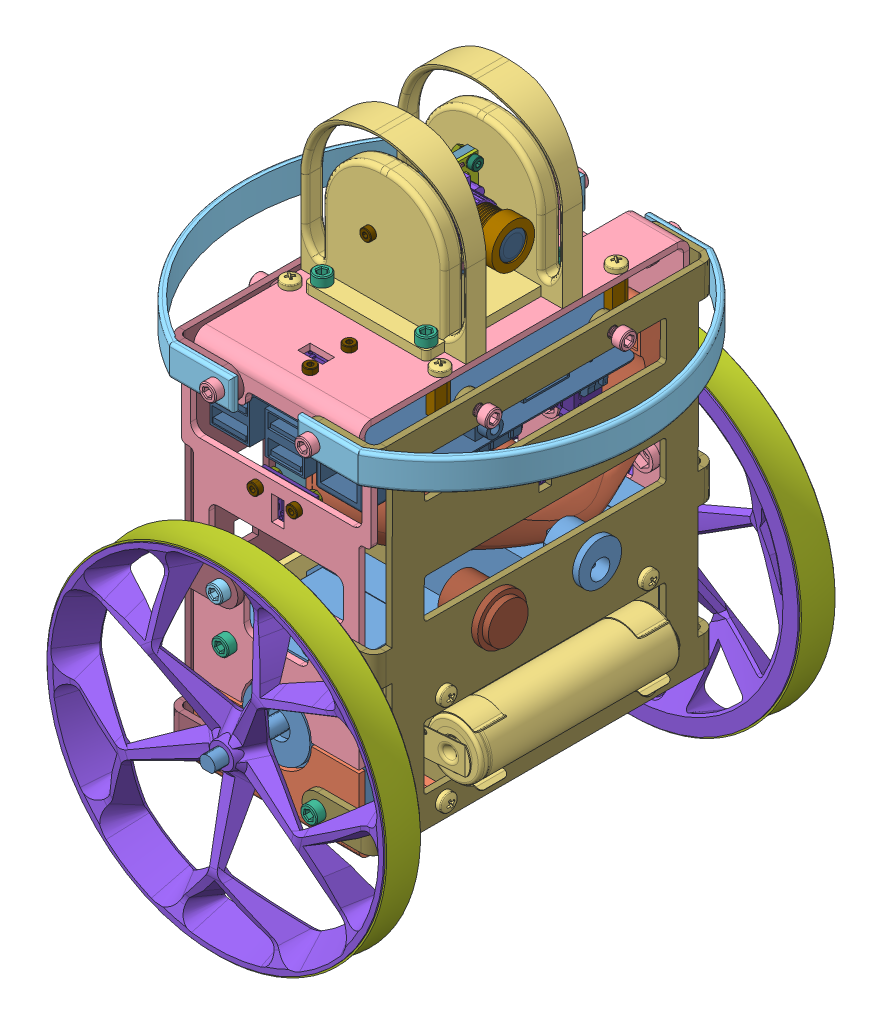
SolidWorks assembly irys5.1, configuration Domyślna. Lengths in mm.
Overall size (135.25 209.52 156.93).
165 component instances, 39 part files, 147 mates.
Components (placement in the parent):
- steppermotor-1: steppermotor [Default] at (-42.2578 -7.1789 72.25) size (42.3 42.3 64.5)
- bottomframe_rys3-1: bottomframe_rys3 [Domyślna] at (-43.1924 -30.5373 18.7182) x (0 0 -1) z (0 -1 0) size (108 54 24.86)
- steppermotor-2: steppermotor [Default] at (-42.2578 -7.1789 -31.75) x (-1 0 0) z (0 0 -1) size (42.3 42.3 64.5)
- battery_module-1: battery_module [Domyślna] at (-62.2578 -30.5373 65.25) x (0 0 -1) z (0 -1 0) size (90 40 22.7)
- topframe-1: topframe [Domyślna] at (-43.6117 88.6087 10.8622) x (0 0 -1) z (0 1 0) size (108 62 97.29)
- bumper-2: bumper [Domyślna] at (-72.7578 82.3211 20.318) x (0 0 1) z (0 -1 0) size (116 57.13 10)
- bumper-3: bumper [Domyślna] at (-11.7578 82.3211 20.25) x (0 0 1) z (0 1 0) size (116 57.13 10)
- imu-1: imu [Domyślna] at (-53.5985 -9.4799 25.3181) x (-0.019519 0 -0.999809) z (0 -1 0) size (10.16 22.86 2.23)
- camera_mounted-1: camera_mounted [Domyślna] at (-50.1687 110.2904 16.7879) x (0 0 -1) z (0.999935 0.011413 0) size (26.1 24.65 29.88)
  - Camera Module Assem-1: Camera Module Assem [Default] at (-12.4357 -13.5775 -13.0743) size (25 24 24.98)
    - PCB 1-1: PCB 1 [Default] at (8.9736 12.851 19.5114) size (25 24 2.1)
    - Camera Block-1: Camera Block [Default] at (8.9736 15.851 20.5114) size (22 13.5 12.5)
    - Camera end-1: Camera end [Default] at (8.9736 15.851 27.3922) x (0.999924 0.012337 0) z (0 0 1) size (14 14 17.26)
    - Lenz-1: Lenz [Default] at (8.9736 15.851 43.8922) size (9 9 0.5)
    - 15 Pin Ribbon Block Assem-1: 15 Pin Ribbon Block Assem [Default] at (0.7567 20.5462 10.9417) x (1 0 0) z (0 -1 0) size (22 2.5 7)
      - 15 Pin Ribbon Block-1: 15 Pin Ribbon Block [Default] at (8.217 10.8197 14.6952) size (20 2.5 6)
      - Ribbon Clamp-1: Ribbon Clamp [Default] at (8.217 10.8197 14.6952) size (22 2.5 5)
    - 0603 Resistor-1: 0603 Resistor [Default] at (2.3268 23.572 20.4882) size (1.75 0.89 0.66)
    - 0603 Resistor-2: 0603 Resistor [Default] at (4.5768 23.572 20.4882) size (1.75 0.89 0.66)
    - 0603 Resistor-3: 0603 Resistor [Default] at (15.6203 23.5707 20.4857) size (1.75 0.89 0.66)
    - 0603 Resistor-4: 0603 Resistor [Default] at (13.3703 23.5707 20.4857) size (1.75 0.89 0.66)
  - mount-1: mount [Domyślna] at (-15.8432 -12.9016 1.4371) size (25 24 5)
  - M2 x 0.4mm Thread 5mm LONG SOCKET HEAD CAP SCREW-1: M2 x 0.4mm Thread 5mm LONG SOCKET HEAD CAP SCREW [Domyślna] at (7.0379 9.2735 2.5371) x (-0.356462 0.93431 0) z (0 0 -1) size (3.8 3.8 7.09)
  - M2 x 0.4mm Thread 5mm LONG SOCKET HEAD CAP SCREW-2: M2 x 0.4mm Thread 5mm LONG SOCKET HEAD CAP SCREW [Domyślna] at (7.0379 -4.7265 2.5371) x (-0.994039 0.109029 0) z (0 0 -1) size (3.8 3.8 7.09)
  - M2 x 0.4mm Thread 5mm LONG SOCKET HEAD CAP SCREW-3: M2 x 0.4mm Thread 5mm LONG SOCKET HEAD CAP SCREW [Domyślna] at (-13.9621 9.2735 2.5371) x (-0.583934 -0.811801 0) z (0 0 -1) size (3.8 3.8 7.09)
  - M2 x 0.4mm Thread 5mm LONG SOCKET HEAD CAP SCREW-4: M2 x 0.4mm Thread 5mm LONG SOCKET HEAD CAP SCREW [Domyślna] at (-13.9621 -4.7265 2.5371) x (-0.923728 -0.383049 0) z (0 0 -1) size (3.8 3.8 7.09)
  - m2_x_0_4mm_thread_hex_nut-1: m2_x_0_4mm_thread_hex_nut [Domyślna] at (7.0379 9.2735 3.1371) size (4 4.62 1.6)
  - m2_x_0_4mm_thread_hex_nut-2: m2_x_0_4mm_thread_hex_nut [Domyślna] at (7.0379 -4.7265 3.1371) size (4 4.62 1.6)
  - m2_x_0_4mm_thread_hex_nut-3: m2_x_0_4mm_thread_hex_nut [Domyślna] at (-13.9621 -4.7265 3.1371) size (4 4.62 1.6)
  - m2_x_0_4mm_thread_hex_nut-4: m2_x_0_4mm_thread_hex_nut [Domyślna] at (-13.9621 9.2735 3.1371) size (4 4.62 1.6)
- ToF_nut-3: ToF_nut [Domyślna] at (-29.7647 53.9524 20.8423) x (0 1 0) z (1 0 0) size (12.89 18.5 4.22)
  - vl53l1x-1: vl53l1x [Domyślna] at (-6.7913 -9.4823 16.6745) size (12.7 17.78 2.22)
  - m2_x_0_4mm_thread_hex_nut-1: m2_x_0_4mm_thread_hex_nut [Domyślna] at (3.3687 5.7577 15.8745) size (4 4.62 1.6)
  - m2_x_0_4mm_thread_hex_nut-2: m2_x_0_4mm_thread_hex_nut [Domyślna] at (3.3687 -6.9423 15.8745) x (-0.923728 -0.383049 0) z (0 0 -1) size (4 4.62 1.6)
  - m2_x_0_4mm_thread_hex_nut-3: m2_x_0_4mm_thread_hex_nut [Domyślna] at (3.3687 5.7577 18.4945) x (-0.923728 -0.383049 0) z (0 0 -1) size (4 4.62 1.6) (hidden)
  - m2_x_0_4mm_thread_hex_nut-4: m2_x_0_4mm_thread_hex_nut [Domyślna] at (3.3687 -6.9423 18.4945) x (-0.923728 -0.383049 0) z (0 0 -1) size (4 4.62 1.6) (hidden)
- m2_x_0_4mm_thread_6mm_long_sock-3: m2_x_0_4mm_thread_6mm_long_sock [Domyślna] at (-14.4701 57.3211 13.9) x (0 0.924225 0.381849) z (-1 0 0) size (3.8 3.8 8)
- m2_x_0_4mm_thread_6mm_long_sock-5: m2_x_0_4mm_thread_6mm_long_sock [Domyślna] at (-14.4701 57.3211 26.6) x (0 0.924225 0.381849) z (-1 0 0) size (3.8 3.8 8)
- ToF_nut-5: ToF_nut [Domyślna] at (-42.1264 69.3142 59.6577) x (1 0 0) z (0 1 0) size (12.89 18.5 4.22)
  - vl53l1x-1: vl53l1x [Domyślna] at (-6.7913 -9.4823 16.6745) size (12.7 17.78 2.22)
  - m2_x_0_4mm_thread_hex_nut-1: m2_x_0_4mm_thread_hex_nut [Domyślna] at (3.3687 5.7577 15.8745) size (4 4.62 1.6)
  - m2_x_0_4mm_thread_hex_nut-2: m2_x_0_4mm_thread_hex_nut [Domyślna] at (3.3687 -6.9423 15.8745) x (-0.923728 -0.383049 0) z (0 0 -1) size (4 4.62 1.6)
  - m2_x_0_4mm_thread_hex_nut-3: m2_x_0_4mm_thread_hex_nut [Domyślna] at (3.3687 5.7577 18.4945) x (-0.923728 -0.383049 0) z (0 0 -1) size (4 4.62 1.6) (hidden)
  - m2_x_0_4mm_thread_hex_nut-4: m2_x_0_4mm_thread_hex_nut [Domyślna] at (3.3687 -6.9423 18.4945) x (-0.923728 -0.383049 0) z (0 0 -1) size (4 4.62 1.6) (hidden)
- m2_x_0_4mm_thread_6mm_long_sock-7: m2_x_0_4mm_thread_6mm_long_sock [Domyślna] at (-38.7578 84.6087 53.9) x (-0.868702 0 -0.495335) z (0 -1 0) size (3.8 3.8 8)
- ToF_nut-6: ToF_nut [Domyślna] at (-42.3452 53.9524 52.9555) x (0 1 0) z (0 0 1) size (12.89 18.5 4.22)
  - vl53l1x-1: vl53l1x [Domyślna] at (-6.7913 -9.4823 16.6745) size (12.7 17.78 2.22)
  - m2_x_0_4mm_thread_hex_nut-1: m2_x_0_4mm_thread_hex_nut [Domyślna] at (3.3687 5.7577 15.8745) size (4 4.62 1.6)
  - m2_x_0_4mm_thread_hex_nut-2: m2_x_0_4mm_thread_hex_nut [Domyślna] at (3.3687 -6.9423 15.8745) x (-0.923728 -0.383049 0) z (0 0 -1) size (4 4.62 1.6)
  - m2_x_0_4mm_thread_hex_nut-3: m2_x_0_4mm_thread_hex_nut [Domyślna] at (3.3687 5.7577 18.4945) x (-0.923728 -0.383049 0) z (0 0 -1) size (4 4.62 1.6) (hidden)
  - m2_x_0_4mm_thread_hex_nut-4: m2_x_0_4mm_thread_hex_nut [Domyślna] at (3.3687 -6.9423 18.4945) x (-0.923728 -0.383049 0) z (0 0 -1) size (4 4.62 1.6) (hidden)
- ToF_nut-7: ToF_nut [Domyślna] at (-41.1605 53.9524 -12.4555) x (0 1 0) z (0 0 -1) size (12.89 18.5 4.22)
  - vl53l1x-1: vl53l1x [Domyślna] at (-6.7913 -9.4823 16.6745) size (12.7 17.78 2.22)
  - m2_x_0_4mm_thread_hex_nut-1: m2_x_0_4mm_thread_hex_nut [Domyślna] at (3.3687 5.7577 15.8745) size (4 4.62 1.6)
  - m2_x_0_4mm_thread_hex_nut-2: m2_x_0_4mm_thread_hex_nut [Domyślna] at (3.3687 -6.9423 15.8745) x (-0.923728 -0.383049 0) z (0 0 -1) size (4 4.62 1.6)
  - m2_x_0_4mm_thread_hex_nut-3: m2_x_0_4mm_thread_hex_nut [Domyślna] at (3.3687 5.7577 18.4945) x (-0.923728 -0.383049 0) z (0 0 -1) size (4 4.62 1.6) (hidden)
  - m2_x_0_4mm_thread_hex_nut-4: m2_x_0_4mm_thread_hex_nut [Domyślna] at (3.3687 -6.9423 18.4945) x (-0.923728 -0.383049 0) z (0 0 -1) size (4 4.62 1.6) (hidden)
- ToF_nut-9: ToF_nut [Domyślna] at (-54.7508 53.9524 -12.3215) x (0 1 0) z (-1 0 0) size (12.89 18.5 4.22)
  - vl53l1x-1: vl53l1x [Domyślna] at (-6.7913 -9.4823 16.6745) size (12.7 17.78 2.22)
  - m2_x_0_4mm_thread_hex_nut-1: m2_x_0_4mm_thread_hex_nut [Domyślna] at (3.3687 5.7577 15.8745) size (4 4.62 1.6)
  - m2_x_0_4mm_thread_hex_nut-2: m2_x_0_4mm_thread_hex_nut [Domyślna] at (3.3687 -6.9423 15.8745) x (-0.923728 -0.383049 0) z (0 0 -1) size (4 4.62 1.6)
  - m2_x_0_4mm_thread_hex_nut-3: m2_x_0_4mm_thread_hex_nut [Domyślna] at (3.3687 5.7577 18.4945) x (-0.923728 -0.383049 0) z (0 0 -1) size (4 4.62 1.6) (hidden)
  - m2_x_0_4mm_thread_hex_nut-4: m2_x_0_4mm_thread_hex_nut [Domyślna] at (3.3687 -6.9423 18.4945) x (-0.923728 -0.383049 0) z (0 0 -1) size (4 4.62 1.6) (hidden)
- m2_x_0_4mm_thread_6mm_long_sock-11: m2_x_0_4mm_thread_6mm_long_sock [Domyślna] at (-69.6779 57.3211 -18.0792) x (0 -0.924225 -0.381849) z (1 0 0) size (3.8 3.8 8)
- m2_x_0_4mm_thread_6mm_long_sock-12: m2_x_0_4mm_thread_6mm_long_sock [Domyślna] at (-69.902 57.3211 -5.3792) x (0 -0.924225 -0.381849) z (1 0 0) size (3.8 3.8 8)
- m2_x_0_4mm_thread_6mm_long_sock-15: m2_x_0_4mm_thread_6mm_long_sock [Domyślna] at (-48.1029 57.3211 68.25) x (-0.262854 -0.964836 0) z (0 0 -1) size (3.8 3.8 8)
- m2_x_0_4mm_thread_6mm_long_sock-16: m2_x_0_4mm_thread_6mm_long_sock [Domyślna] at (-35.4029 57.3211 68.25) x (0.638921 -0.769272 0) z (0 0 -1) size (3.8 3.8 8)
- m2_x_0_4mm_thread_6mm_long_sock-17: m2_x_0_4mm_thread_6mm_long_sock [Domyślna] at (-48.1029 57.3211 -27.75) size (3.8 3.8 8)
- m2_x_0_4mm_thread_6mm_long_sock-18: m2_x_0_4mm_thread_6mm_long_sock [Domyślna] at (-35.9963 57.335 -27.7658) size (3.8 3.8 8)
- H-H_M3x12mm-1: H-H_M3x12mm [Predeterminado] at (-51.2078 -22.4959 17.65) x (0.837169 0 0.546944) z (0.546944 0 -0.837169) size (5.77 12 5)
- H-H_M3x6mm-1: H-H_M3x6mm [Predeterminado] at (-51.2078 -13.4959 17.65) x (0.837169 0 0.546944) z (0.546944 0 -0.837169) size (5.77 6 5)
- pan cross head_am-2: pan cross head_am [B18.6.7M - M3 x 0.5 x 6 Type I Cross Recessed PHMS --6N] at (-51.2078 -7.0799 17.65) x (0 -1 0) z (0 0 1) size (8.37 5.6 5.6)
- battery_module_H-2: battery_module_H [Domyślna] at (13.655 -6.0808 19.8906) x (0 0 1) z (-1 0 0) size (90 40 24.06)
  - battery_module-1: battery_module [Domyślna] at (-44.6406 -21.0981 81.7004) size (90 40 22.7)
  - H-H_M3x6mm-1: H-H_M3x6mm [Predeterminado] at (-32.6406 13.9019 84.7004) x (1 0 0) z (0 1 0) size (5.77 6 5)
  - H-H_M3x6mm-2: H-H_M3x6mm [Predeterminado] at (33.3594 13.9019 84.7004) x (1 0 0) z (0 1 0) size (5.77 6 5)
  - H-H_M3x6mm-3: H-H_M3x6mm [Predeterminado] at (-32.6406 -16.0981 84.7004) x (1 0 0) z (0 -1 0) size (5.77 6 5)
  - H-H_M3x6mm-4: H-H_M3x6mm [Predeterminado] at (33.3594 -16.0981 84.7004) x (1 0 0) z (0 1 0) size (5.77 6 5)
  - pan cross head_am-1: pan cross head_am [B18.6.7M - M3 x 0.5 x 6 Type I Cross Recessed PHMS --6N] at (-32.6406 -16.0981 77.2589) x (0 0 1) z (-1 0 0) size (8.37 5.6 5.6)
  - pan cross head_am-3: pan cross head_am [B18.6.7M - M3 x 0.5 x 6 Type I Cross Recessed PHMS --6N] at (-32.6406 13.9019 77.2589) x (0 0 1) z (-1 0 0) size (8.37 5.6 5.6)
  - pan cross head_am-4: pan cross head_am [B18.6.7M - M3 x 0.5 x 6 Type I Cross Recessed PHMS --6N] at (33.3594 13.9019 77.2589) x (0 0 1) z (-1 0 0) size (8.37 5.6 5.6)
  - pan cross head_am-5: pan cross head_am [B18.6.7M - M3 x 0.5 x 6 Type I Cross Recessed PHMS --6N] at (33.3594 -16.0981 77.2589) x (0 0 1) z (-1 0 0) size (8.37 5.6 5.6)
- pan cross head_am-3: pan cross head_am [B18.6.7M - M3 x 0.5 x 6 Type I Cross Recessed PHMS --6N] at (-78.4454 -22.1789 53.25) size (8.37 5.6 5.6)
- pan cross head_am-4: pan cross head_am [B18.6.7M - M3 x 0.5 x 6 Type I Cross Recessed PHMS --6N] at (-78.4454 7.8211 53.25) size (8.37 5.6 5.6)
- pan cross head_am-5: pan cross head_am [B18.6.7M - M3 x 0.5 x 6 Type I Cross Recessed PHMS --6N] at (-78.4454 7.8211 -12.75) size (8.37 5.6 5.6)
- pan cross head_am-6: pan cross head_am [B18.6.7M - M3 x 0.5 x 6 Type I Cross Recessed PHMS --6N] at (-78.4454 -22.1789 -12.75) size (8.37 5.6 5.6)
- pan cross head_am-7: pan cross head_am [B18.6.7M - M3 x 0.5 x 6 Type I Cross Recessed PHMS --6N] at (-57.2578 -34.9373 53.25) x (0 1 0) z (0 0 1) size (8.37 5.6 5.6)
- pan cross head_am-8: pan cross head_am [B18.6.7M - M3 x 0.5 x 6 Type I Cross Recessed PHMS --6N] at (-27.2578 -34.9373 53.25) x (0 1 0) z (0 0 1) size (8.37 5.6 5.6)
- pan cross head_am-9: pan cross head_am [B18.6.7M - M3 x 0.5 x 6 Type I Cross Recessed PHMS --6N] at (-57.2578 -34.9373 -12.75) x (0 1 0) z (0 0 1) size (8.37 5.6 5.6)
- pan cross head_am-10: pan cross head_am [B18.6.7M - M3 x 0.5 x 6 Type I Cross Recessed PHMS --6N] at (-27.2578 -34.9373 -12.75) x (0 1 0) z (0 0 1) size (8.37 5.6 5.6)
- battery_module_H-3: battery_module_H [Domyślna] at (-98.1705 -8.277 19.8906) x (0 0 1) z (1 0 0) size (90 40 24.06)
  - battery_module-1: battery_module [Domyślna] at (-44.6406 -21.0981 81.7004) size (90 40 22.7)
  - H-H_M3x6mm-1: H-H_M3x6mm [Predeterminado] at (-32.6406 13.9019 84.7004) x (1 0 0) z (0 1 0) size (5.77 6 5)
  - H-H_M3x6mm-2: H-H_M3x6mm [Predeterminado] at (33.3594 13.9019 84.7004) x (1 0 0) z (0 1 0) size (5.77 6 5)
  - H-H_M3x6mm-3: H-H_M3x6mm [Predeterminado] at (-32.6406 -16.0981 84.7004) x (1 0 0) z (0 -1 0) size (5.77 6 5)
  - H-H_M3x6mm-4: H-H_M3x6mm [Predeterminado] at (33.3594 -16.0981 84.7004) x (1 0 0) z (0 1 0) size (5.77 6 5)
  - pan cross head_am-1: pan cross head_am [B18.6.7M - M3 x 0.5 x 6 Type I Cross Recessed PHMS --6N] at (-32.6406 -16.0981 77.2589) x (0 0 1) z (-1 0 0) size (8.37 5.6 5.6)
  - pan cross head_am-3: pan cross head_am [B18.6.7M - M3 x 0.5 x 6 Type I Cross Recessed PHMS --6N] at (-32.6406 13.9019 77.2589) x (0 0 1) z (-1 0 0) size (8.37 5.6 5.6)
  - pan cross head_am-4: pan cross head_am [B18.6.7M - M3 x 0.5 x 6 Type I Cross Recessed PHMS --6N] at (33.3594 13.9019 77.2589) x (0 0 1) z (-1 0 0) size (8.37 5.6 5.6)
  - pan cross head_am-5: pan cross head_am [B18.6.7M - M3 x 0.5 x 6 Type I Cross Recessed PHMS --6N] at (33.3594 -16.0981 77.2589) x (0 0 1) z (-1 0 0) size (8.37 5.6 5.6)
- pan cross head_am-11: pan cross head_am [B18.6.7M - M3 x 0.5 x 6 Type I Cross Recessed PHMS --6N] at (-6.0701 -22.1789 53.25) x (-1 0 0) z (0 0.924225 0.381849) size (8.37 5.6 5.6)
- pan cross head_am-12: pan cross head_am [B18.6.7M - M3 x 0.5 x 6 Type I Cross Recessed PHMS --6N] at (-6.0701 7.8211 53.25) x (-1 0 0) z (0 0.924225 0.381849) size (8.37 5.6 5.6)
- pan cross head_am-13: pan cross head_am [B18.6.7M - M3 x 0.5 x 6 Type I Cross Recessed PHMS --6N] at (-6.0701 7.8211 -12.75) x (-1 0 0) z (0 0.924225 0.381849) size (8.37 5.6 5.6)
- pan cross head_am-14: pan cross head_am [B18.6.7M - M3 x 0.5 x 6 Type I Cross Recessed PHMS --6N] at (-6.0701 -22.1789 -12.75) x (-1 0 0) z (0 0.924225 0.381849) size (8.37 5.6 5.6)
- M3x6-1: M3x6 [Default] at (-57.7578 82.3211 -40.75) x (0 0 1) z (0.923728 0.383049 0) size (9 5.5 5.5)
- M3x6-2: M3x6 [Default] at (-26.7578 82.3211 -40.75) x (0 0 1) z (0.923728 0.383049 0) size (9 5.5 5.5)
- M3x4-1: M3x4 [Default] at (-26.7578 24.3211 -38.75) x (0 0 1) z (0.923728 0.383049 0) size (7 5.5 5.5)
- M3x4-2: M3x4 [Default] at (-57.7578 24.3211 -38.75) x (0 0 1) z (0.923728 0.383049 0) size (7 5.5 5.5)
- M3x8-1: M3x8 [Default] at (-26.7578 8.3211 -36.75) x (0 0 1) z (0.923728 0.383049 0) size (9 5.5 5.5)
- M3x8-2: M3x8 [Default] at (-57.7578 8.3211 -36.75) x (0 0 1) z (0.923728 0.383049 0) size (9 5.5 5.5)
- M3x8-3: M3x8 [Default] at (-26.7578 -22.6789 -38.75) x (0 0 1) z (-0.923728 -0.383049 0) size (9 5.5 5.5)
- M3x8-4: M3x8 [Default] at (-57.7578 -22.6789 -38.75) x (0 0 1) z (0.923728 0.383049 0) size (9 5.5 5.5)
- M3x6-3: M3x6 [Default] at (-57.7578 82.3211 81.318) x (0 0 -1) z (-0.923728 -0.383049 0) size (9 5.5 5.5)
- M3x6-4: M3x6 [Default] at (-26.7578 82.3211 81.25) x (0 0 -1) z (-0.923728 -0.383049 0) size (9 5.5 5.5)
- M3x4-3: M3x4 [Default] at (-57.7578 24.3211 79.25) x (0 0 -1) z (-0.923728 -0.383049 0) size (7 5.5 5.5)
- M3x4-4: M3x4 [Default] at (-26.7578 24.3211 79.25) x (0 0 -1) z (-0.923728 -0.383049 0) size (7 5.5 5.5)
- M3x8-5: M3x8 [Default] at (-57.7578 8.3211 77.25) x (0 0 -1) z (-0.923728 -0.383049 0) size (9 5.5 5.5)
- M3x8-6: M3x8 [Default] at (-26.7578 8.3211 77.25) x (0 0 -1) z (-0.923728 -0.383049 0) size (9 5.5 5.5)
- M3x8-7: M3x8 [Default] at (-57.7578 -22.6789 79.25) x (0 0 -1) z (-0.923728 -0.383049 0) size (9 5.5 5.5)
- M3x8-8: M3x8 [Default] at (-26.7578 -22.6789 79.25) x (0 0 -1) z (-0.923728 -0.383049 0) size (9 5.5 5.5)
- wheel_module-1: wheel_module [Domyślna] at (-153.2578 -13.8345 -56.9103) x (0 0 1) z (1 0 0) size (16.77 112.94 112.94)
  - tire wide-1: tire wide [Domyślna] at (-0.6464 -6.6556 111) size (11 111 111)
  - wheel_rim_minirys-1: wheel_rim_minirys [Domyślna] at (15.6603 -6.6556 111) x (0 0.027139 0.999632) z (-1 0 0) size (110 110 16.77)
- wheel_module-2: wheel_module [Domyślna] at (-153.4368 -5.0545 97.8035) x (0 0 -1) z (0.999168 0.040772 0) size (16.77 112.94 112.94)
  - tire wide-1: tire wide [Domyślna] at (-0.6464 -6.6556 111) size (11 111 111)
  - wheel_rim_minirys-1: wheel_rim_minirys [Domyślna] at (15.6603 -6.6556 111) x (0 0.027139 0.999632) z (-1 0 0) size (110 110 16.77)
- m2_x_0_4mm_thread_6mm_long_sock-19: m2_x_0_4mm_thread_6mm_long_sock [Domyślna] at (-38.7578 84.6087 66.6) x (-0.868702 0 -0.495335) z (0 -1 0) size (3.8 3.8 8)
- M3x6-5: M3x6 [Default] at (-80.7156 82.8211 -1.75) x (1 0 0) z (0 -0.999999 0.001298) size (9 5.5 5.5)
- M3x6-6: M3x6 [Default] at (-80.685 82.8211 42.25) x (1 0 0) z (0 -0.999999 0.001298) size (9 5.5 5.5)
- M3x6-7: M3x6 [Default] at (-3.0454 82.8211 42.25) x (-1 0 0) z (0 -0.383049 0.923728) size (9 5.5 5.5)
- M3x6-8: M3x6 [Default] at (-3.0454 82.8211 -1.75) x (-1 0 0) z (0 -0.383049 0.923728) size (9 5.5 5.5)
- H-M_M3x10x6mm-1: H-M_M3x10x6mm [Predeterminado] at (-66.7578 78.6087 45.25) size (5.77 16 5)
- H-M_M3x10x6mm-2: H-M_M3x10x6mm [Predeterminado] at (-18.2481 78.6087 45.3511) size (5.77 16 5)
- H-M_M3x10x6mm-5: H-M_M3x10x6mm [Predeterminado] at (-66.7578 78.6087 -12.7875) size (5.77 16 5)
- H-M_M3x10x6mm-6: H-M_M3x10x6mm [Predeterminado] at (-18.2481 78.6087 -12.6864) size (5.77 16 5)
- rys_PCB_rpi_simple-2: rys_PCB_rpi_simple [Domyślna] at (-94.7865 65.3087 -58.1904) x (1 0 0) z (0 -1 0) size (61.22 87.74 23.25)
- pan cross head_am-15: pan cross head_am [B18.6.7M - M3 x 0.5 x 6 Type I Cross Recessed PHMS --6N] at (-66.7578 93.0087 45.25) x (0 -1 0) z (-0.546944 0 0.837169) size (8.37 5.6 5.6)
- pan cross head_am-16: pan cross head_am [B18.6.7M - M3 x 0.5 x 6 Type I Cross Recessed PHMS --6N] at (-18.1875 93.0087 -12.75) x (0 -1 0) z (-0.546944 0 0.837169) size (8.37 5.6 5.6)
- pan cross head_am-17: pan cross head_am [B18.6.7M - M3 x 0.5 x 6 Type I Cross Recessed PHMS --6N] at (-66.7578 93.0087 -12.75) x (0 -1 0) z (-0.546944 0 0.837169) size (8.37 5.6 5.6)
- pan cross head_am-18: pan cross head_am [B18.6.7M - M3 x 0.5 x 6 Type I Cross Recessed PHMS --6N] at (-17.7578 93.0087 45.25) x (0 -1 0) z (-0.546944 0 0.837169) size (8.37 5.6 5.6)
- switch_simple-1: switch_simple [Domyślna] at (-4.4701 21.3211 36.25) x (0 0 1) z (-1 0 0) size (16 16 16)
- frontv5-4: frontv5 [Domyślna] at (-10.3534 69.423 20.4236) x (0 0 -1) z (-0.002586 -0.999997 0) size (112 23.29 115)
- frontv2.1-1: frontv2.1 [Domyślna] at (-74.0454 69.4652 20.0972) x (0 0 1) z (0 -1 0) size (112 23.29 115)
- fan_simple_2-6: fan_simple_2 [Domyślna] at (-74.0454 35.3211 20.2708) x (0 -1 0) z (0 0 1) size (45 10 45)
- M3x20-1: M3x20 [Default] at (-79.0454 16.8211 38.7708) size (23.05 5.5 5.5)
- M3x20-2: M3x20 [Default] at (-79.0454 16.8211 1.7708) size (23.05 5.5 5.5)
- M3x20-3: M3x20 [Default] at (-79.0454 53.8211 1.7708) size (23.05 5.5 5.5)
- M3x20-4: M3x20 [Default] at (-79.0454 53.8211 38.7708) size (23.05 5.5 5.5)
- M3_NUT-1: M3_NUT [Valor predeterminado] at (-60.7954 16.8211 38.7969) x (0 0 -1) z (1 0 0) size (6.55 5.4 2.5)
- M3_NUT-2: M3_NUT [Valor predeterminado] at (-60.9756 16.7949 1.797) x (0 0 -1) z (1 0 0) size (6.55 5.4 2.5)
- M3_NUT-3: M3_NUT [Valor predeterminado] at (-60.8582 53.7949 1.7708) x (0 0 -1) z (1 0 0) size (6.55 5.4 2.5)
- M3_NUT-4: M3_NUT [Valor predeterminado] at (-60.7954 53.8211 38.7708) x (0 0 -1) z (1 0 0) size (6.55 5.4 2.5)
- 430250200.stp-4: 430250200.stp [Domyślna] at (-24.9794 51.5777 -9.5364) x (-0.999962 0 -0.008727) z (0.008727 0 -0.999962) size (5.28 14 10.85)
- 430250200.stp-5: 430250200.stp [Domyślna] at (-40.3519 51.7087 -9.9151) x (-0.999962 0 -0.008727) z (0.008727 0 -0.999962) size (5.28 14 10.85)
- 430250200.stp-6: 430250200.stp [Domyślna] at (-47.7794 51.7087 -9.6936) x (-0.999962 0 -0.008727) z (0.008727 0 -0.999962) size (5.28 14 10.85)
- 430250200.stp-7: 430250200.stp [Domyślna] at (-31.8678 51.7087 -9.7603) x (-0.999962 0 -0.008727) z (0.008727 0 -0.999962) size (5.28 14 10.85)
- M2 x 0.4mm Thread 10mm LONG SOCKET HEAD CAP SCREW-5: M2 x 0.4mm Thread 10mm LONG SOCKET HEAD CAP SCREW [Domyślna] at (-46.2578 112.6087 11.25) x (-0.266188 0.963921 0) z (0 0 1) size (3.8 3.8 12.09)
- M2 x 0.4mm Thread 10mm LONG SOCKET HEAD CAP SCREW-6: M2 x 0.4mm Thread 10mm LONG SOCKET HEAD CAP SCREW [Domyślna] at (-46.2578 112.6087 29.25) x (-0.999935 -0.011413 0) z (0 0 -1) size (3.8 3.8 12.09)
- M3x8-9: M3x8 [Default] at (-25.2578 96.6087 -1.75) x (0 -1 0) z (-0.923728 0 0.383049) size (9 5.5 5.5)
- M3x8-13: M3x8 [Default] at (-59.2578 96.6087 42.25) x (0 -1 0) z (-0.923728 0 0.383049) size (9 5.5 5.5)
- M3x8-14: M3x8 [Default] at (-25.2578 96.6087 42.25) x (0 -1 0) z (-0.923728 0 0.383049) size (9 5.5 5.5)
- M3x8-15: M3x8 [Default] at (-59.2578 96.6087 -1.75) x (0 -1 0) z (-0.923728 0 0.383049) size (9 5.5 5.5)
- Panel_Mount_2mm_Power_Plug_v2.step-1: Panel_Mount_2mm_Power_Plug_v2.step [Domyślna] at (-6.4714 21.2686 4.25) x (0 -0.000012 -1) z (0.002586 0.999997 -0.000012) size (14 13.69 14)
- tunelv3.2-1: tunelv3.2 [Domyślna] at (-62.0454 58.4238 13.3551) x (0 -0.000707 -1) z (1 0 0) size (74.54 69.73 61.73)
- mount3-1: mount3 [Domyślna] at (-42.2578 90.6087 20.25) x (0 0 -1) z (1 0 0) size (50 53 54.12)
Mates (geometry in assembly coordinates):
- Koncentryczne1: concentric aligned: cylinder of steppermotor-1 through (-26.7578 -22.6789 64.75) axis (0 0 1) radius 1.25; cylinder of bottomframe_rys3-1 through (-26.7578 -22.6789 74.25) axis (0 0 1) radius 1.6
- Koncentryczne2: concentric aligned: cylinder of steppermotor-1 through (-57.7578 -22.6789 64.75) axis (0 0 1) radius 1.25; cylinder of bottomframe_rys3-1 through (-57.7578 -22.6789 74.25) axis (0 0 1) radius 1.6
- Wspólnie1: coincident anti-aligned: plane of steppermotor-1 through (-64.2538 -29.1749 72.25) normal (0 0 1); plane of bottomframe_rys3-1 through (-42.2578 -7.6789 72.25) normal (0 0 -1)
- Koncentryczne3: concentric aligned: cylinder of bottomframe_rys3-1 through (-57.7578 -22.6789 -33.75) axis (0 0 -1) radius 1.6; cylinder of steppermotor-2 through (-57.7578 -22.6789 -24.25) axis (0 0 -1) radius 1.25
- Koncentryczne4: concentric aligned: circle of bottomframe_rys3-1; cylinder of steppermotor-2 through (-26.7578 -22.6789 -24.25) axis (0 0 -1) radius 1.25
- Wspólnie2: coincident anti-aligned: plane of bottomframe_rys3-1 through (-42.2578 -159.6789 -31.75) normal (0 0 1); plane of steppermotor-2 through (-20.2618 -29.1749 -31.75) normal (0 0 -1)
- Koncentryczne7: concentric aligned: cylinder of steppermotor-2 through (-26.7578 8.3211 -24.25) axis (0 0 -1) radius 1.25; cylinder of topframe-1 through (-26.7578 8.3211 -33.75) axis (0 0 -1) radius 1.6
- Koncentryczne8: concentric aligned: cylinder of steppermotor-1 through (-57.7578 8.3211 64.75) axis (0 0 1) radius 1.25; cylinder of topframe-1 through (-57.7578 8.3211 74.25) axis (0 0 1) radius 1.6
- Wspólnie4: coincident anti-aligned: plane of steppermotor-1 through (-64.2538 -29.1749 72.25) normal (0 0 1); plane of topframe-1 through (-70.7578 55.8211 72.25) normal (0 0 -1)
- Koncentryczne18: concentric aligned: cylinder of bottomframe_rys3-1 through (-26.7578 -22.6789 -33.75) axis (0 0 -1) radius 1.6; cylinder of steppermotor-2 through (-26.7578 -22.6789 -24.25) axis (0 0 -1) radius 1.25
- Koncentryczne36: concentric aligned: cylinder of topframe-1 through (-57.7578 82.3211 74.25) axis (0 0 1) radius 1.6; cylinder of bumper-2 through (-57.7578 82.3211 -37.682) axis (0 0 1) radius 1.5
- Koncentryczne37: concentric aligned: cylinder of topframe-1 through (-26.7578 82.3211 74.25) axis (0 0 1) radius 1.6; cylinder of bumper-3 through (-26.7578 82.3211 -37.75) axis (0 0 1) radius 1.5
- Koncentryczne55: concentric aligned: cylinder of battery_module-1 through (-51.2078 -28.4959 17.65) axis (0 1 0) radius 1.1; cylinder of imu-1 through (-51.2078 -10.4959 17.65) axis (0 1 0) radius 1.0922
- Koncentryczne56: concentric anti-aligned: cylinder of bottomframe_rys3-1 through (-27.2578 -32.5373 53.25) axis (0 -1 0) radius 1.4; cylinder of battery_module-1 through (-27.2578 -28.4959 53.25) axis (0 1 0) radius 1.6
- Koncentryczne57: concentric anti-aligned: cylinder of bottomframe_rys3-1 through (-57.2578 -32.5373 -12.75) axis (0 -1 0) radius 1.4; cylinder of battery_module-1 through (-57.2578 -28.4959 -12.75) axis (0 1 0) radius 1.6
- Wspólnie27: coincident anti-aligned: plane of bottomframe_rys3-1 through (-42.2578 -30.5373 96.25) normal (0 1 0); plane of battery_module-1 through (-62.2578 -30.5373 65.25) normal (0 -1 0)
- Koncentryczne63: concentric aligned: cylinder of topframe-1 through (-38.7578 90.6087 4.6) axis (0 1 0) radius 1.25; cylinder of camera_mounted-1/mount1-1 through (-38.7578 90.6087 4.6) axis (0 1 0) radius 1.05
- Koncentryczne65: concentric aligned: cylinder of topframe-1 through (-38.7578 90.6087 35.9) axis (0 1 0) radius 1.25; cylinder of camera_mounted-1/mount1-1 through (-38.7578 90.6087 35.9) axis (0 1 0) radius 1.05
- Wspólnie34: coincident anti-aligned: plane of topframe-1 through (-70.7578 90.6087 105.75) normal (0 1 0); plane of camera_mounted-1/mount1-1 through (-41.7578 90.6087 2.1027) normal (0 -1 0)
- Wspólnie61: coincident anti-aligned: plane of topframe-1 through (-70.7578 88.6087 105.75) normal (0 -1 0); plane of ToF_nut-5/m2_x_0_4mm_thread_hex_nut-4 through (-37.3526 88.6087 64.7673) normal (0 1 0)
- Koncentryczne100: concentric anti-aligned: cylinder of camera_mounted-1/mount1-1 through (-38.7578 90.6087 35.9) axis (0 1 0) radius 1.05; cylinder of M2 x 0.4mm Thread 10mm LONG SOCKET HEAD CAP SCREW-4 through (-38.7578 95.6087 35.9) axis (0 -1 0) radius 1.9
- Wspólnie64: coincident anti-aligned: plane of camera_mounted-1/mount1-1 through (-41.7578 93.6087 7.7527) normal (0 1 0); plane of M2 x 0.4mm Thread 10mm LONG SOCKET HEAD CAP SCREW-4 through (-38.7578 93.6087 35.9) normal (0 -1 0)
- Koncentryczne104: concentric aligned: cylinder of topframe-1 through (-38.7578 90.6087 53.9) axis (0 1 0) radius 1.25; cylinder of m2_x_0_4mm_thread_6mm_long_sock-7 through (-38.7578 92.6087 53.9) axis (0 1 0) radius 1.9
- Wspólnie65: coincident anti-aligned: plane of topframe-1 through (-70.7578 90.6087 105.75) normal (0 1 0); plane of m2_x_0_4mm_thread_6mm_long_sock-7 through (-38.7578 90.6087 53.9) normal (0 -1 0)
- Wspólnie67: coincident anti-aligned: plane of topframe-1 through (-70.7578 55.8211 72.25) normal (0 0 -1); plane of ToF_nut-6/m2_x_0_4mm_thread_hex_nut-4 through (-37.2356 58.7262 72.25) normal (0 0 1)
- Wspólnie68: coincident anti-aligned: plane of topframe-1 through (-70.7578 226.8211 -31.75) normal (0 0 1); plane of ToF_nut-7/m2_x_0_4mm_thread_hex_nut-3 through (-33.5701 58.7262 -31.75) normal (0 0 -1)
- Wspólnie78: coincident anti-aligned: plane of topframe-1 through (-70.7578 55.8211 74.25) normal (0 0 1); plane of m2_x_0_4mm_thread_6mm_long_sock-15 through (-48.1029 57.3211 74.25) normal (0 0 -1)
- Wspólnie79: coincident anti-aligned: plane of topframe-1 through (-70.7578 55.8211 74.25) normal (0 0 1); plane of m2_x_0_4mm_thread_6mm_long_sock-16 through (-35.4029 57.3211 74.25) normal (0 0 -1)
- Wspólnie80: coincident anti-aligned: plane of topframe-1 through (-70.7578 226.8211 -33.75) normal (0 0 -1); plane of m2_x_0_4mm_thread_6mm_long_sock-17 through (-48.1029 57.3211 -33.75) normal (0 0 1)
- Koncentryczne125: concentric aligned: cylinder of battery_module-1 through (-51.2078 -28.4959 17.65) axis (0 1 0) radius 1.1; cylinder of H-H_M3x12mm-1 through (-51.2078 -28.4959 17.65) axis (0 1 0) radius 1.5
- Wspólnie82: coincident anti-aligned: plane of battery_module-1 through (-62.2578 -28.4959 65.25) normal (0 1 0); plane of H-H_M3x12mm-1 through (-51.2078 -28.4959 17.65) normal (0 -1 0)
- Wspólnie83: coincident anti-aligned: circle of H-H_M3x12mm-1; cylinder of H-H_M3x6mm-1 through (-51.2078 -16.4959 17.65) axis (0 1 0) radius 1.5
- Wspólnie84: coincident anti-aligned: plane of H-H_M3x12mm-1 through (-51.2078 -16.4959 17.65) normal (0 1 0); plane of H-H_M3x6mm-1 through (-51.2078 -16.4959 17.65) normal (0 -1 0)
- Wspólnie85: coincident anti-aligned: plane of imu-1 through (-53.5985 -10.4959 25.3181) normal (0 -1 0); plane of H-H_M3x6mm-1 through (-51.2078 -10.4959 17.65) normal (0 1 0)
- Koncentryczne1261: concentric aligned: cylinder of imu-1 through (-51.2078 -10.4959 17.65) axis (0 1 0) radius 1.0922; cylinder of pan cross head_am-2 through (-51.2078 18.3201 17.65) axis (0 1 0) radius 2.8
- Wspólnie871: coincident anti-aligned: plane of imu-1 through (-53.5985 -9.4799 25.3181) normal (0 1 0); plane of pan cross head_am-2 through (-49.7078 -9.4799 17.65) normal (0 -1 0)
- Koncentryczne1331: concentric aligned: cylinder of bottomframe_rys3-1 through (-57.2578 -32.5373 53.25) axis (0 -1 0) radius 1.4; cylinder of pan cross head_am-7 through (-57.2578 -60.3373 53.25) axis (0 -1 0) radius 2.8
- Wspólnie931: coincident anti-aligned: plane of bottomframe_rys3-1 through (-42.2578 -32.5373 96.25) normal (0 -1 0); plane of pan cross head_am-7 through (-58.7578 -32.5373 53.25) normal (0 1 0)
- Koncentryczne1341: concentric aligned: cylinder of bottomframe_rys3-1 through (-27.2578 -32.5373 53.25) axis (0 -1 0) radius 1.4; cylinder of pan cross head_am-8 through (-27.2578 -60.3373 53.25) axis (0 -1 0) radius 2.8
- Wspólnie941: coincident anti-aligned: plane of bottomframe_rys3-1 through (-42.2578 -32.5373 96.25) normal (0 -1 0); plane of pan cross head_am-8 through (-28.7578 -32.5373 53.25) normal (0 1 0)
- Koncentryczne1351: concentric aligned: cylinder of bottomframe_rys3-1 through (-57.2578 -32.5373 -12.75) axis (0 -1 0) radius 1.4; cylinder of pan cross head_am-9 through (-57.2578 -60.3373 -12.75) axis (0 -1 0) radius 2.8
- Wspólnie951: coincident anti-aligned: plane of bottomframe_rys3-1 through (-42.2578 -32.5373 96.25) normal (0 -1 0); plane of pan cross head_am-9 through (-58.7578 -32.5373 -12.75) normal (0 1 0)
- Koncentryczne1361: concentric aligned: cylinder of bottomframe_rys3-1 through (-27.2578 -32.5373 -12.75) axis (0 -1 0) radius 1.4; cylinder of pan cross head_am-10 through (-27.2578 -60.3373 -12.75) axis (0 -1 0) radius 2.8
- Wspólnie961: coincident anti-aligned: plane of bottomframe_rys3-1 through (-42.2578 -32.5373 96.25) normal (0 -1 0); plane of pan cross head_am-10 through (-28.7578 -32.5373 -12.75) normal (0 1 0)
- Wspólnie104: coincident anti-aligned: plane of bumper-3 through (-31.7578 77.3211 -37.75) normal (0 0 -1); plane of M3x6-2 through (-26.187 80.9447 -37.75) normal (0 0 1)
- Koncentryczne148: concentric aligned: cylinder of topframe-1 through (-26.7578 8.3211 -33.75) axis (0 0 -1) radius 1.6; cylinder of M3x8-1 through (-26.7578 8.3211 -125.4555) axis (0 0 -1) radius 2.75
- Wspólnie107: coincident anti-aligned: plane of topframe-1 through (-70.7578 226.8211 -33.75) normal (0 0 -1); plane of M3x8-1 through (-26.187 6.9447 -33.75) normal (0 0 1)
- Koncentryczne149: concentric aligned: cylinder of topframe-1 through (-57.7578 8.3211 -33.75) axis (0 0 -1) radius 1.6; cylinder of M3x8-2 through (-57.7578 8.3211 -125.4555) axis (0 0 -1) radius 2.75
- Wspólnie108: coincident anti-aligned: plane of topframe-1 through (-70.7578 226.8211 -33.75) normal (0 0 -1); plane of M3x8-2 through (-57.187 6.9447 -33.75) normal (0 0 1)
- Koncentryczne150: concentric aligned: cylinder of bottomframe_rys3-1 through (-57.7578 -22.6789 -33.75) axis (0 0 -1) radius 1.6; cylinder of M3x8-4 through (-57.7578 -22.6789 -127.4555) axis (0 0 -1) radius 2.75
- Koncentryczne153: concentric aligned: circle of topframe-1; cylinder of M3x6-3 through (-57.7578 82.3211 170.0235) axis (0 0 1) radius 2.75
- Wspólnie112: coincident anti-aligned: plane of bumper-2 through (-73.1394 87.3211 78.318) normal (0 0 1); plane of M3x6-3 through (-57.187 80.9447 78.318) normal (0 0 -1)
- Koncentryczne155: concentric aligned: cylinder of topframe-1 through (-57.7578 24.3211 74.25) axis (0 0 1) radius 1.6; cylinder of M3x4-3 through (-57.7578 24.3211 167.9555) axis (0 0 1) radius 2.75
- Koncentryczne158: concentric aligned: cylinder of topframe-1 through (-26.7578 8.3211 74.25) axis (0 0 1) radius 1.6; cylinder of M3x8-6 through (-26.7578 8.3211 165.9555) axis (0 0 1) radius 2.75
- Koncentryczne159: concentric aligned: cylinder of topframe-1 through (-57.7578 8.3211 74.25) axis (0 0 1) radius 1.6; cylinder of M3x8-5 through (-57.7578 8.3211 165.9555) axis (0 0 1) radius 2.75
- Wspólnie115: coincident anti-aligned: plane of topframe-1 through (-70.7578 55.8211 74.25) normal (0 0 1); plane of M3x8-5 through (-57.187 6.9447 74.25) normal (0 0 -1)
- Wspólnie116: coincident anti-aligned: plane of topframe-1 through (-70.7578 55.8211 74.25) normal (0 0 1); plane of M3x8-6 through (-26.187 6.9447 74.25) normal (0 0 -1)
- Koncentryczne1447: concentric aligned: cylinder of topframe-1 through (-48.1029 57.3211 -33.75) axis (0 0 1) radius 1.25; cylinder of ToF_nut-7/vl53l1x-1 through (-48.1029 57.3211 -30.15) axis (0 0 1) radius 1.0922
- Koncentryczne1448: concentric aligned: cylinder of topframe-1 through (-35.4029 57.3211 -33.75) axis (0 0 1) radius 1.25; cylinder of ToF_nut-7/vl53l1x-1 through (-35.4029 57.3211 -30.15) axis (0 0 1) radius 1.0922
- Równolegle1: parallel aligned: plane of ToF_nut-7/m2_x_0_4mm_thread_hex_nut-1 through (-34.2482 55.3211 -27.53) normal (0 0 1); plane of m2_x_0_4mm_thread_6mm_long_sock-18 through (-35.9963 57.335 -33.7658) normal (0 0 1)
- Koncentryczne1454: concentric aligned: circle of topframe-1; circle of ToF_nut-6/m2_x_0_4mm_thread_hex_nut-3
- Koncentryczne1455: concentric aligned: circle of topframe-1; circle of ToF_nut-6/m2_x_0_4mm_thread_hex_nut-4
- Koncentryczne1456: concentric aligned: circle of topframe-1; circle of m2_x_0_4mm_thread_6mm_long_sock-16
- Koncentryczne1457: concentric aligned: circle of topframe-1; circle of m2_x_0_4mm_thread_6mm_long_sock-15
- Koncentryczne1458: concentric aligned: circle of topframe-1; circle of m2_x_0_4mm_thread_6mm_long_sock-17
- Koncentryczne1461: concentric anti-aligned: circle of topframe-1; cylinder of ToF_nut-5/vl53l1x-1 through (-38.7578 87.0087 53.9) axis (0 -1 0) radius 1.0922
- Koncentryczne1462: concentric aligned: circle of topframe-1; circle of m2_x_0_4mm_thread_6mm_long_sock-19
- Koncentryczne1463: concentric anti-aligned: circle of bumper2-1; circle of M3x6-7
- Wspólnie970: coincident anti-aligned: plane of bumper2-1 through (-6.0454 102.864 47.0753) normal (1 0 0); plane of M3x6-7 through (-6.0454 81.4447 41.6793) normal (-1 0 0)
- Koncentryczne1464: concentric anti-aligned: circle of bumper2-2; circle of M3x6-8
- Wspólnie971: coincident anti-aligned: plane of bumper2-2 through (-6.0454 102.864 3.0753) normal (1 0 0); plane of M3x6-8 through (-6.0454 81.4447 -2.3207) normal (-1 0 0)
- Koncentryczne1465: concentric aligned: circle of bumper2-1; circle of M3x6-6
- Koncentryczne1466: concentric aligned: circle of bumper2-2; circle of M3x6-5
- Koncentryczne1483: concentric aligned: circle of H-M_M3x10x6mm-1; circle of rys_PCB_rpi_simple-2
- Wspólnie978: coincident anti-aligned: plane of H-M_M3x10x6mm-1 through (-66.7578 78.6087 45.25) normal (0 -1 0); plane of rys_PCB_rpi_simple-2 through (-42.2266 78.6087 26.4747) normal (0 1 0)
- Koncentryczne1484: concentric aligned: circle of H-M_M3x10x6mm-2; circle of rys_PCB_rpi_simple-2
- Wspólnie979: coincident anti-aligned: plane of H-M_M3x10x6mm-2 through (-18.2481 78.6087 45.3511) normal (0 -1 0); plane of rys_PCB_rpi_simple-2 through (-42.2266 78.6087 26.4747) normal (0 1 0)
- Koncentryczne1485: concentric aligned: circle of H-M_M3x10x6mm-5; circle of rys_PCB_rpi_simple-2
- Wspólnie980: coincident anti-aligned: plane of H-M_M3x10x6mm-5 through (-66.7578 78.6087 -12.7875) normal (0 -1 0); plane of rys_PCB_rpi_simple-2 through (-42.2266 78.6087 26.4747) normal (0 1 0)
- Koncentryczne1486: concentric aligned: circle of H-M_M3x10x6mm-6; circle of rys_PCB_rpi_simple-2
- Wspólnie981: coincident anti-aligned: plane of H-M_M3x10x6mm-6 through (-18.2481 78.6087 -12.6864) normal (0 -1 0); plane of rys_PCB_rpi_simple-2 through (-42.2266 78.6087 26.4747) normal (0 1 0)
- Koncentryczne1487: concentric anti-aligned: circle of topframe-1; circle of H-M_M3x10x6mm-1
- Wspólnie982: coincident anti-aligned: plane of topframe-1 through (-70.7578 88.6087 105.75) normal (0 -1 0); plane of H-M_M3x10x6mm-1 through (-66.7578 88.6087 45.25) normal (0 1 0)
- Koncentryczne1490: concentric aligned: circle of topframe-1; circle of M3X6_PLASTIC-2
- Wspólnie983: coincident aligned: plane of topframe-1 through (-70.7578 90.6087 105.75) normal (0 1 0); circle of M3X6_PLASTIC-2
- Koncentryczne1491: concentric aligned: circle of topframe-1; circle of M3X6_PLASTIC-3
- Wspólnie985: coincident aligned: plane of topframe-1 through (-70.7578 90.6087 105.75) normal (0 1 0); circle of M3X6_PLASTIC-3
- Koncentryczne1492: concentric aligned: circle of topframe-1; circle of M3X6_PLASTIC-1
- Wspólnie986: coincident aligned: plane of topframe-1 through (-70.7578 90.6087 105.75) normal (0 1 0); circle of M3X6_PLASTIC-1
- Koncentryczne1493: concentric aligned: circle of topframe-1; circle of M3X6_PLASTIC-4
- Wspólnie987: coincident aligned: plane of topframe-1 through (-70.7578 90.6087 105.75) normal (0 1 0); circle of M3X6_PLASTIC-4
- Stycznie1: tangent: circle of topframe-1; circle of front-4
- Koncentryczne1502: concentric aligned: circle of topframe-1; circle of front-4
- Koncentryczne1506: concentric aligned: circle of bottomframe_rys3-1; circle of frontv2-1
- Koncentryczne1507: concentric aligned: circle of topframe-1; circle of frontv2-1
- Koncentryczne1509: concentric aligned: circle of frontv2-1; circle of fan_simple-6
- Wspólnie1003: coincident anti-aligned: plane of frontv2.1-1 through (-74.0454 82.3211 -50.7292) normal (1 0 0); plane of fan_simple_2-6 through (-74.0454 54.8211 39.7708) normal (-1 0 0)
- Wspólnie1004: coincident anti-aligned: circle of fan_simple-6; circle of tunel-2
- Koncentryczne1514: concentric aligned: circle of frontv2-1; circle of M3x20-3
- Koncentryczne1515: concentric aligned: circle of frontv2-1; circle of M3x20-4
- Koncentryczne1516: concentric aligned: circle of frontv2-1; circle of M3x20-1
- Koncentryczne1517: concentric aligned: circle of frontv2-1; circle of M3x20-2
- Wspólnie1005: coincident anti-aligned: circle of tunel-2; circle of M3_NUT-1
- Wspólnie1006: coincident anti-aligned: circle of tunel-2; circle of M3_NUT-2
- Wspólnie1007: coincident anti-aligned: circle of tunel-2; circle of M3_NUT-4
- Wspólnie1009: coincident anti-aligned: circle of tunel-2; circle of M3_NUT-3
- Koncentryczne1518: concentric aligned: circle of steppermotor-2; circle of wheel_module-1/wheel_rim_minirys-1
- Wspólnie1010: coincident anti-aligned: plane of steppermotor-2 through (-43.8633 -9.0734 -41.25) normal (0 0 -1); plane of wheel_module-1/wheel_rim_minirys-1 through (-42.2578 -7.1789 -41.25) normal (0 0 1)
- Wspólnie1011: coincident anti-aligned: plane of frontv2.1-1 through (-76.0454 82.3211 -50.7292) normal (-1 0 0); plane of M3x20-3 through (-76.0454 55.3111 1.7708) normal (1 0 0)
- Wspólnie1012: coincident anti-aligned: plane of frontv2.1-1 through (-76.0454 82.3211 -50.7292) normal (-1 0 0); plane of M3x20-4 through (-76.0454 55.3111 38.7708) normal (1 0 0)
- Wspólnie1013: coincident anti-aligned: plane of frontv2.1-1 through (-76.0454 82.3211 -50.7292) normal (-1 0 0); plane of M3x20-1 through (-76.0454 18.3111 38.7708) normal (1 0 0)
- Wspólnie1014: coincident anti-aligned: plane of frontv2.1-1 through (-76.0454 82.3211 -50.7292) normal (-1 0 0); plane of M3x20-2 through (-76.0454 18.3111 1.7708) normal (1 0 0)
- Wspólnie1015: coincident anti-aligned: plane of topframe-1 through (-70.7578 90.6087 105.75) normal (0 1 0); plane of m2_x_0_4mm_thread_6mm_long_sock-19 through (-38.7578 90.6087 66.6) normal (0 -1 0)
- Równolegle8: parallel anti-aligned: plane of rys_PCB_rpi_simple-2 through (-27.3114 55.3587 -6.0403) normal (0 -1 0); plane of 430250200.stp-4 through (-26.9343 55.2277 -6.1233) normal (0 1 0)
- Wspólnie1024: coincident anti-aligned: plane of rys_PCB_rpi_simple-2 through (-50.9865 55.3587 -6.0153) normal (0 -1 0); plane of 430250200.stp-6 through (-49.7342 55.3587 -6.2806) normal (0 1 0)
- Wspólnie1025: coincident anti-aligned: plane of rys_PCB_rpi_simple-2 through (-43.1115 55.3587 -6.0153) normal (0 -1 0); plane of 430250200.stp-5 through (-42.3068 55.3587 -6.5021) normal (0 1 0)
- Wspólnie1026: coincident anti-aligned: plane of rys_PCB_rpi_simple-2 through (-35.2115 55.3587 -6.0153) normal (0 -1 0); plane of 430250200.stp-7 through (-33.8227 55.3587 -6.3472) normal (0 1 0)
- Koncentryczne1524: concentric aligned: circle of mount2-1; circle of M3x8-13
- Wspólnie1031: coincident anti-aligned: plane of mount2-1 through (-60.7578 93.6087 -3.25) normal (0 1 0); plane of M3x8-13 through (-58.687 93.6087 43.6264) normal (0 -1 0)
- Koncentryczne1525: concentric aligned: circle of mount2-1; circle of M3x8-14
- Koncentryczne1526: concentric aligned: circle of mount2-1; circle of M3x8-15
- Koncentryczne1527: concentric aligned: circle of mount2-1; circle of M3x8-9
- Wspólnie1032: coincident aligned: plane of mount2-1 through (-60.7578 93.6087 -3.25) normal (0 1 0); circle of M3x8-14
- Wspólnie1033: coincident aligned: plane of mount2-1 through (-60.7578 93.6087 -3.25) normal (0 1 0); circle of M3x8-15
- Wspólnie1034: coincident anti-aligned: plane of mount2-1 through (-60.7578 93.6087 -3.25) normal (0 1 0); plane of M3x8-9 through (-24.687 93.6087 -0.3736) normal (0 -1 0)
- Koncentryczne1531: concentric anti-aligned: circle of mount2-1; circle of M2 x 0.4mm Thread 10mm LONG SOCKET HEAD CAP SCREW-6
- Wspólnie1036: coincident anti-aligned: plane of mount2-1 through (-42.2578 133.6087 39.25) normal (0 0 1); plane of M2 x 0.4mm Thread 10mm LONG SOCKET HEAD CAP SCREW-6 through (-52.2578 111.1087 39.25) normal (0 0 -1)
- Koncentryczne1532: concentric anti-aligned: circle of camera_mounted-1/mount-1; circle of mount2-1
- Koncentryczne1533: concentric aligned: circle of mount2-1; circle of M2 x 0.4mm Thread 10mm LONG SOCKET HEAD CAP SCREW-5
- Wspólnie1038: coincident anti-aligned: plane of mount2-1 through (-42.2578 133.6087 1.25) normal (0 0 -1); plane of M2 x 0.4mm Thread 10mm LONG SOCKET HEAD CAP SCREW-5 through (-46.2578 111.6936 1.25) normal (0 0 1)
- Wspólnie1039: coincident anti-aligned: circle of fan_simple-6; circle of tunelv3-2
- Koncentryczne1534: concentric anti-aligned: circle of front-4; circle of Panel_Mount_2mm_Power_Plug_v2.step-1
- Wspólnie1040: coincident anti-aligned: plane of frontv5-4 through (-8.3202 82.2736 91.25) normal (0.999997 -0.002586 0); circle of Panel_Mount_2mm_Power_Plug_v2.step-1
- Wspólnie1041: coincident anti-aligned: circle of fan_simple-6; circle of tunelv3.1-1
- Wspólnie1042: coincident aligned: circle of frontv2.1-1; circle of fan_simple_2-6
- Koncentryczne1535: concentric aligned: cylinder of m2_x_0_4mm_thread_6mm_long_sock-11 through (-77.6779 57.3211 -18.0792) axis (-1 0 0) radius 1.9; circle of frontv2.1-1
- Koncentryczne1536: concentric anti-aligned: circle of m2_x_0_4mm_thread_6mm_long_sock-12; circle of frontv2.1-1
- Koncentryczne1537: concentric anti-aligned: circle of ToF_nut-9/m2_x_0_4mm_thread_hex_nut-4; circle of frontv2.1-1
- Koncentryczne1538: concentric aligned: circle of M3_NUT-4; circle of tunelv3.2-1
- Koncentryczne1539: concentric aligned: circle of M3_NUT-3; circle of tunelv3.2-1
- Koncentryczne1540: concentric aligned: circle of M3_NUT-1; circle of tunelv3.2-1
- Koncentryczne1541: concentric aligned: circle of M3_NUT-2; circle of tunelv3.2-1
- Koncentryczne1542: concentric aligned: circle of M2 x 0.4mm Thread 10mm LONG SOCKET HEAD CAP SCREW-5; circle of mount3-1
- Koncentryczne1543: concentric aligned: circle of topframe-1; cylinder of mount3-1 through (-25.2578 90.6087 42.25) axis (0 1 0) radius 1.35
- Wspólnie1048: coincident anti-aligned: plane of topframe-1 through (-70.7578 90.6087 105.75) normal (0 1 0); plane of mount3-1 through (-60.7578 90.6087 -3.25) normal (0 -1 0)
- Koncentryczne1548: concentric aligned: circle of M2 x 0.4mm Thread 10mm LONG SOCKET HEAD CAP SCREW-6; circle of mount3-1
- Wspólnie1049: coincident aligned: circle of camera_mounted-1/mount-1; circle of mount3-1
